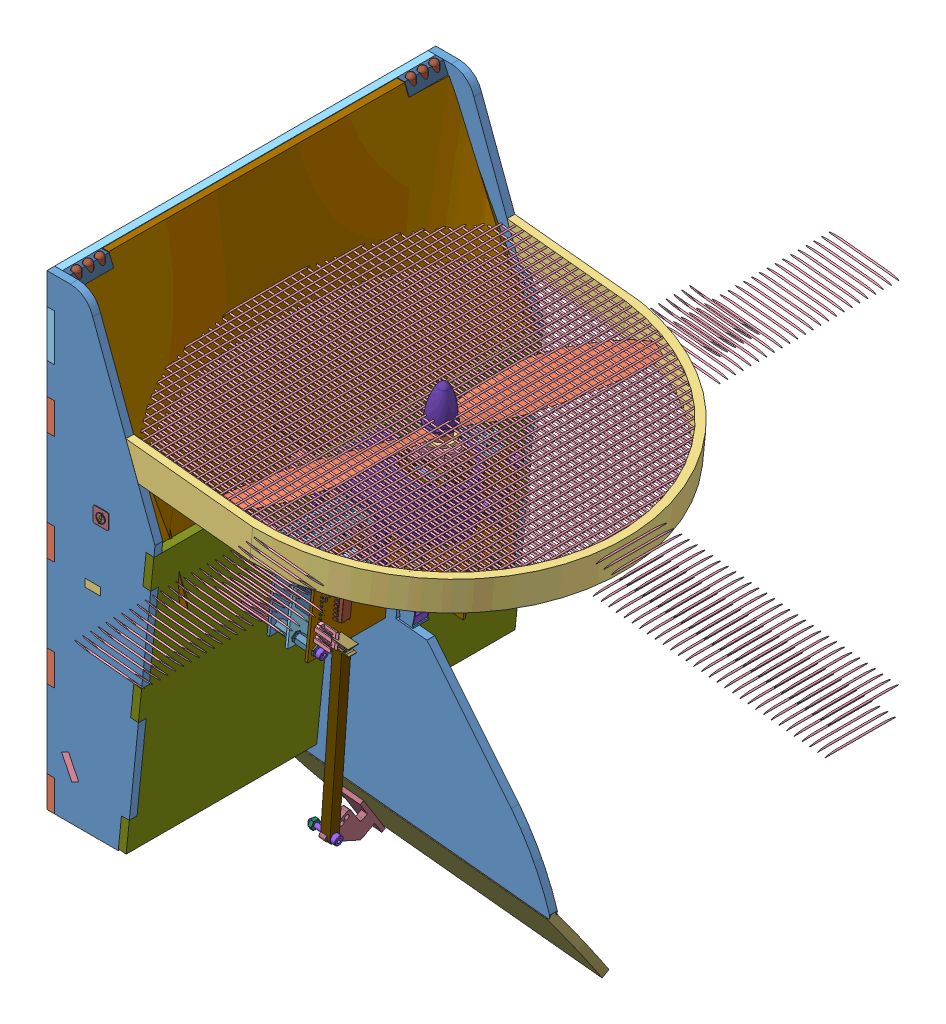
SolidWorks assembly AssTotaleSimu7, configuration Défaut. Lengths in mm. (continued)
Components (placement in the parent): (continued)
- AssStructSimu-1: AssStructSimu [Défaut] at (-125.7658 -1.8483 624.6548) x (1 0 0) z (0 0 -1) size (253.25 324.59 251.6) (continued)
  - AssCarte-1: AssCarte [Défaut] at (38.0121 147.1029 290.772) x (-0.101852 0.9948 0) z (0.9948 0.101852 0) size (66.52 130.57 98.72) (continued)
    - carte_onduleur_v3-1: carte_onduleur_v3 [Défaut] at (-131.8199 12.0892 20.7912) size (66.52 130.57 82.34) (continued)
      - RC2_2-1: RC2_2 [Défaut] at (-22 0.18 -0.803) x (-1 0 0) z (0 0 -1) size (2.34 1.04 0.5) (continued)
        - Open CASCADE STEP translator 6.8 1.12.1-1: Open CASCADE STEP translator 6.8 1.12.1 [Défaut] at origin size (2.34 1.04 0.5) (continued)
          - Pin_2_2-1: Pin_2_2 [Défaut] at origin size (0.51 1.02 0.5)
      - RC3_1-1: RC3_1 [Défaut] at (-20.9336 -14.5 -0.803) x (1 0 0) z (0 0 -1) size (2.34 1.04 0.5)
        - Open CASCADE STEP translator 6.8 1.12.1-1: Open CASCADE STEP translator 6.8 1.12.1 [Défaut] at origin size (2.34 1.04 0.5)
          - Body_1_3-1: Body_1_3 [Défaut] at origin size (2.29 1.04 0.43)
          - Pin_1_2-1: Pin_1_2 [Défaut] at (0.3048 0 0) x (-1 0 0) z (0 0 1) size (0.51 1.02 0.5)
          - Pin_2_2-1: Pin_2_2 [Défaut] at origin size (0.51 1.02 0.5)
      - RC3_2-1: RC3_2 [Défaut] at (-22.3 -14.5 -0.803) x (-1 0 0) z (0 0 -1) size (2.34 1.04 0.5)
        - Open CASCADE STEP translator 6.8 1.12.1-1: Open CASCADE STEP translator 6.8 1.12.1 [Défaut] at origin size (2.34 1.04 0.5)
          - Body_1_3-1: Body_1_3 [Défaut] at origin size (2.29 1.04 0.43)
          - Pin_1_2-1: Pin_1_2 [Défaut] at (0.3048 0 0) x (-1 0 0) z (0 0 1) size (0.51 1.02 0.5)
          - Pin_2_2-1: Pin_2_2 [Défaut] at origin size (0.51 1.02 0.5)
      - U_MES_CUR-1: U_MES_CUR [Défaut] at (-11.5 6.7816 0.803) size (2.54 2.41 0.76)
        - Open CASCADE STEP translator 6.8 1.32.1-1: Open CASCADE STEP translator 6.8 1.32.1 [Défaut] at origin size (2.54 2.41 0.76)
          - Body_1_5-1: Body_1_5 [Défaut] at origin size (2.54 1.27 0.71)
          - Pin_1_3-1: Pin_1_3 [Défaut] at (-2.1082 0.2286 0) x (0 -1 0) z (0 0 1) size (1.14 0.25 0.47)
          - Pin_2_3-1: Pin_2_3 [Défaut] at (-0.2032 2.1336 0) x (0 -1 0) z (0 0 1) size (1.14 0.25 0.47)
      - CARTE_ALIM-1: CARTE_ALIM [Défaut] at (-6.4 -57.2 0.803) size (60 130 18.35)
        - Open CASCADE STEP translator 6.8 1.33.1-1: Open CASCADE STEP translator 6.8 1.33.1 [Défaut] at origin size (60 130 18.35)
          - Body_1_6-1: Body_1_6 [Défaut] at (7 56 -12) size (60 130 18.35)
            - 1_3-1: 1_3 [Défaut] at origin size (60 130 1.61)
            - 13_3-1: 13_3 [Défaut] at (0.4717 -40.93 0.803) x (0 1 0) z (0 0 1) size (5.65 4.9 1.7)
              - =_[0_1_1_4]_3-1: =_[0_1_1_4]_3 [Défaut] at origin size (5.65 4.9 1.7)
                - 2-1: 2 [Défaut] at origin size (3.75 4.9 1.53)
                - 3-1: 3 [Défaut] at origin size (0.95 0.51 1.06)
                - 4-1: 4 [Défaut] at origin size (0.95 0.51 1.06)
                - 5_2-1: 5_2 [Défaut] at origin size (0.95 0.51 1.06)
                - 6-1: 6 [Défaut] at origin size (0.95 0.51 1.06)
                - 7-1: 7 [Défaut] at (10.8 -5.08 0) x (-1 0 0) z (0 0 1) size (0.95 0.51 1.06)
                - 8_2-1: 8_2 [Défaut] at (10.8 -2.54 0) x (-1 0 0) z (0 0 1) size (0.95 0.51 1.06)
                - 9-1: 9 [Défaut] at (10.8 0 0) x (-1 0 0) z (0 0 1) size (0.95 0.51 1.06)
                - 10-1: 10 [Défaut] at (10.8 2.54 0) x (-1 0 0) z (0 0 1) size (0.95 0.51 1.06)
                - 11_2-1: 11_2 [Défaut] at (5.4 -1.27 0) x (-1 0 0) z (0 0 1) size (4.25 2.34 1.06)
            - 18-1: 18 [Défaut] at (-2.5283 -37.23 0.803) x (0 -1 0) z (0 0 1) size (2.34 1.04 0.5)
              - =_[0_1_1_16]-1: =_[0_1_1_16] [Défaut] at origin size (2.34 1.04 0.5)
                - 14_2-1: 14_2 [Défaut] at origin size (2.29 1.04 0.43)
                - 15_2-1: 15_2 [Défaut] at (0.3048 0 0) x (-1 0 0) z (0 0 1) size (0.51 1.02 0.5)
                - 16_2-1: 16_2 [Défaut] at origin size (0.51 1.02 0.5)
            - 21_2-1: 21_2 [Défaut] at (-2.2263 -24.628 -0.803) x (1 0 0) z (0 0 -1) size (8.01 8 14.24)
              - =_[0_1_1_21]-1: =_[0_1_1_21] [Défaut] at origin size (8.01 8 14.24)
                - 19-1: 19 [Défaut] at (1.8 0 0) x (1 0 0) z (0 -1 0) size (8.01 14.24 8)
            - 23_2-1: 23_2 [Défaut] at (1.2381 -31.53 0.803) size (2.34 1.04 0.5)
              - =_[0_1_1_16]-1: =_[0_1_1_16] [Défaut] at origin size (2.34 1.04 0.5)
                - 14_2-1: 14_2 [Défaut] at origin size (2.29 1.04 0.43)
                - 15_2-1: 15_2 [Défaut] at (0.3048 0 0) x (-1 0 0) z (0 0 1) size (0.51 1.02 0.5)
                - 16_2-1: 16_2 [Défaut] at origin size (0.51 1.02 0.5)
            - 28-1: 28 [Défaut] at (5 29.8636 0.803) x (0 -1 0) z (0 0 1) size (3.35 1.3 0.55)
              - =_[0_1_1_25]_2-1: =_[0_1_1_25]_2 [Défaut] at origin size (3.35 1.3 0.55)
                - 24-1: 24 [Défaut] at origin size (3.3 1.3 0.48)
                - 25_2-1: 25_2 [Défaut] at (0.5588 0 0) x (-1 0 0) z (0 0 1) size (0.76 1.27 0.55)
                - 26_2-1: 26_2 [Défaut] at origin size (0.76 1.27 0.55)
            - 30-1: 30 [Défaut] at (6.7 29.8636 0.803) x (0 -1 0) z (0 0 1) size (2.34 1.04 0.5)
              - =_[0_1_1_16]-1: =_[0_1_1_16] [Défaut] at origin size (2.34 1.04 0.5)
                - 14_2-1: 14_2 [Défaut] at origin size (2.29 1.04 0.43)
                - 15_2-1: 15_2 [Défaut] at (0.3048 0 0) x (-1 0 0) z (0 0 1) size (0.51 1.02 0.5)
                - 16_2-1: 16_2 [Défaut] at origin size (0.51 1.02 0.5)
            - 35_2-1: 35_2 [Défaut] at (-2.5 -46.37 0.803) x (0 1 0) z (0 0 1) size (3.4 2.06 0.79)
              - =_[0_1_1_31]-1: =_[0_1_1_31] [Défaut] at origin size (3.4 2.06 0.79)
                - 31_2-1: 31_2 [Défaut] at origin size (3.3 2.06 0.69)
                - 32_3-1: 32_3 [Défaut] at (0.5588 0 0) x (-1 0 0) z (0 0 1) size (0.81 2.03 0.79)
                - 33_3-1: 33_3 [Défaut] at origin size (0.81 2.03 0.79)
            - 37-1: 37 [Défaut] at (5 31.43 0.803) x (0 1 0) z (0 0 1) size (2.34 1.04 0.5)
              - =_[0_1_1_16]-1: =_[0_1_1_16] [Défaut] at origin size (2.34 1.04 0.5)
                - 14_2-1: 14_2 [Défaut] at origin size (2.29 1.04 0.43)
                - 15_2-1: 15_2 [Défaut] at (0.3048 0 0) x (-1 0 0) z (0 0 1) size (0.51 1.02 0.5)
                - 16_2-1: 16_2 [Défaut] at origin size (0.51 1.02 0.5)
            - 39-1: 39 [Défaut] at (-0.2 35.63 0.803) x (-1 0 0) z (0 0 1) size (2.34 1.04 0.5)
              - =_[0_1_1_16]-1: =_[0_1_1_16] [Défaut] at origin size (2.34 1.04 0.5)
                - 14_2-1: 14_2 [Défaut] at origin size (2.29 1.04 0.43)
                - 15_2-1: 15_2 [Défaut] at (0.3048 0 0) x (-1 0 0) z (0 0 1) size (0.51 1.02 0.5)
                - 16_2-1: 16_2 [Défaut] at origin size (0.51 1.02 0.5)
            - 41-1: 41 [Défaut] at (2.9 -45.5036 0.803) x (0 1 0) z (0 0 1) size (2.34 1.04 0.5)
              - =_[0_1_1_16]-1: =_[0_1_1_16] [Défaut] at origin size (2.34 1.04 0.5)
                - 14_2-1: 14_2 [Défaut] at origin size (2.29 1.04 0.43)
                - 15_2-1: 15_2 [Défaut] at (0.3048 0 0) x (-1 0 0) z (0 0 1) size (0.51 1.02 0.5)
                - 16_2-1: 16_2 [Défaut] at origin size (0.51 1.02 0.5)
            - 43-1: 43 [Défaut] at (17.1348 -42.6272 0.803) x (0 1 0) z (0 0 1) size (2.34 1.04 0.5)
              - =_[0_1_1_16]-1: =_[0_1_1_16] [Défaut] at origin size (2.34 1.04 0.5)
                - 14_2-1: 14_2 [Défaut] at origin size (2.29 1.04 0.43)
                - 15_2-1: 15_2 [Défaut] at (0.3048 0 0) x (-1 0 0) z (0 0 1) size (0.51 1.02 0.5)
                - 16_2-1: 16_2 [Défaut] at origin size (0.51 1.02 0.5)
            - 48_2-1: 48_2 [Défaut] at (-5.4717 -39.01 0.803) x (-1 0 0) z (0 0 1) size (4.19 3.4 1.75)
              - =_[0_1_1_40]-1: =_[0_1_1_40] [Défaut] at origin size (4.19 3.4 1.75)
                - 44_2-1: 44_2 [Défaut] at origin size (3.75 3.38 1.73)
                - 45_2-1: 45_2 [Défaut] at (0.438 0 0) x (-1 0 0) z (0 0 1) size (0.53 3.4 1.75)
                - 46_2-1: 46_2 [Défaut] at origin size (0.52 3.4 1.75)
            - 53-1: 53 [Défaut] at (0.9 35.63 0.803) size (2.34 1.04 0.5)
              - =_[0_1_1_45]-1: =_[0_1_1_45] [Défaut] at origin size (2.34 1.04 0.5)
                - 49_3-1: 49_3 [Défaut] at origin size (2.29 1.04 0.43)
                - 50-1: 50 [Défaut] at (0.3048 0 0) x (-1 0 0) z (0 0 1) size (0.51 1.02 0.5)
                - 51-1: 51 [Défaut] at origin size (0.51 1.02 0.5)
            - 55_2-1: 55_2 [Défaut] at (1.3 -45.5036 0.803) x (0 1 0) z (0 0 1) size (2.34 1.04 0.5)
              - =_[0_1_1_45]-1: =_[0_1_1_45] [Défaut] at origin size (2.34 1.04 0.5)
                - 49_3-1: 49_3 [Défaut] at origin size (2.29 1.04 0.43)
                - 50-1: 50 [Défaut] at (0.3048 0 0) x (-1 0 0) z (0 0 1) size (0.51 1.02 0.5)
                - 51-1: 51 [Défaut] at origin size (0.51 1.02 0.5)
            - 57_3-1: 57_3 [Défaut] at (17.2348 -43.9936 0.803) x (0 -1 0) z (0 0 1) size (2.34 1.04 0.5)
              - =_[0_1_1_45]-1: =_[0_1_1_45] [Défaut] at origin size (2.34 1.04 0.5)
                - 49_3-1: 49_3 [Défaut] at origin size (2.29 1.04 0.43)
                - 50-1: 50 [Défaut] at (0.3048 0 0) x (-1 0 0) z (0 0 1) size (0.51 1.02 0.5)
                - 51-1: 51 [Défaut] at origin size (0.51 1.02 0.5)
            - 65-1: 65 [Défaut] at (-4.8 30.93 0.803) x (-1 0 0) z (0 0 1) size (14.64 9.83 4.25)
              - =_[0_1_1_52]-1: =_[0_1_1_52] [Défaut] at origin size (14.64 9.83 4.25)
                - 63_2-1: 63_2 [Défaut] at (3 0 0) x (0 -1 0) z (0 0 1) size (9.83 14.64 4.25)
                  - =_[0_1_1_3]_5-1: =_[0_1_1_3]_5 [Défaut] at origin size (9.83 9.05 4.21)
                  - =_[0_1_1_4]_5-1: =_[0_1_1_4]_5 [Défaut] at origin size (9.48 7.76 1.21)
                  - =_[0_1_1_5]_5-1: =_[0_1_1_5]_5 [Défaut] at origin size (1.36 6.01 3.08)
                  - =_[0_1_1_6]_3-1: =_[0_1_1_6]_3 [Défaut] at origin size (1.36 6.01 3.08)
                  - =_[0_1_1_7]_3-1: =_[0_1_1_7]_3 [Défaut] at origin size (1.06 6.01 3.08)
            - 67-1: 67 [Défaut] at (13.5933 -37.5272 0.803) x (-1 0 0) z (0 0 1) size (2.34 1.04 0.5)
              - =_[0_1_1_16]-1: =_[0_1_1_16] [Défaut] at origin size (2.34 1.04 0.5)
                - 14_2-1: 14_2 [Défaut] at origin size (2.29 1.04 0.43)
                - 15_2-1: 15_2 [Défaut] at (0.3048 0 0) x (-1 0 0) z (0 0 1) size (0.51 1.02 0.5)
                - 16_2-1: 16_2 [Défaut] at origin size (0.51 1.02 0.5)
            - 70_2-1: 70_2 [Défaut] at (18.2733 -29.7272 0.803) x (0 1 0) z (0 0 1) size (6.06 4.95 1.88)
              - =_[0_1_1_61]-1: =_[0_1_1_61] [Défaut] at origin size (6.06 4.95 1.88)
                - 68-1: 68 [Défaut] x (1 0 0) z (0 -1 0) size (6.06 1.88 4.95)
            - 83-1: 83 [Défaut] at (-21.2 -38.07 0.803) x (-1 0 0) z (0 0 1) size (2.7 5.2 1.11)
              - =_[0_1_1_64]-1: =_[0_1_1_64] [Défaut] at origin size (2.7 5.2 1.11)
                - 84_2-1: 84_2 [Défaut] at (1.2 -4 0) x (0 1 0) z (0 0 1) size (5.2 2.7 1.11)
                  - =_[0_1_1_3]_6-1: =_[0_1_1_3]_6 [Défaut] at origin size (0.39 0.64 0.01)
                  - =_[0_1_1_4]_6-1: =_[0_1_1_4]_6 [Défaut] at origin size (0.6 1.9 0.2)
                  - =_[0_1_1_5]_6-1: =_[0_1_1_5]_6 [Défaut] at origin size (0.21 0.08 0.01)
                  - =_[0_1_1_6]_4-1: =_[0_1_1_6]_4 [Défaut] at origin size (0.6 1.9 0.2)
                  - =_[0_1_1_7]_4-1: =_[0_1_1_7]_4 [Défaut] at origin size (0.46 0.68 0.01)
                  - =_[0_1_1_8]_3-1: =_[0_1_1_8]_3 [Défaut] at origin size (0.38 0.66 0.01)
                  - =_[0_1_1_9]_2-1: =_[0_1_1_9]_2 [Défaut] at origin size (0.2 0.62 0.01)
                  - =_[0_1_1_10]_2-1: =_[0_1_1_10]_2 [Défaut] at origin size (4 2.7 1.1)
                  - =_[0_1_1_11]_2-1: =_[0_1_1_11]_2 [Défaut] at origin size (0.46 0.63 0.01)
                  - =_[0_1_1_12]_2-1: =_[0_1_1_12]_2 [Défaut] at origin size (0.56 0.68 0.01)
            - 86_2-1: 86_2 [Défaut] at (12.8933 -35.4272 0.803) x (0 1 0) z (0 0 1) size (2.7 5.2 1.11)
              - =_[0_1_1_77]-1: =_[0_1_1_77] [Défaut] at origin size (2.7 5.2 1.11)
                - 84_2-1: 84_2 [Défaut] at (1.2 -4 0) x (0 1 0) z (0 0 1) size (5.2 2.7 1.11)
                  - =_[0_1_1_3]_6-1: =_[0_1_1_3]_6 [Défaut] at origin size (0.39 0.64 0.01)
                  - =_[0_1_1_4]_6-1: =_[0_1_1_4]_6 [Défaut] at origin size (0.6 1.9 0.2)
                  - =_[0_1_1_5]_6-1: =_[0_1_1_5]_6 [Défaut] at origin size (0.21 0.08 0.01)
                  - =_[0_1_1_6]_4-1: =_[0_1_1_6]_4 [Défaut] at origin size (0.6 1.9 0.2)
                  - =_[0_1_1_7]_4-1: =_[0_1_1_7]_4 [Défaut] at origin size (0.46 0.68 0.01)
                  - =_[0_1_1_8]_3-1: =_[0_1_1_8]_3 [Défaut] at origin size (0.38 0.66 0.01)
                  - =_[0_1_1_9]_2-1: =_[0_1_1_9]_2 [Défaut] at origin size (0.2 0.62 0.01)
                  - =_[0_1_1_10]_2-1: =_[0_1_1_10]_2 [Défaut] at origin size (4 2.7 1.1)
                  - =_[0_1_1_11]_2-1: =_[0_1_1_11]_2 [Défaut] at origin size (0.46 0.63 0.01)
                  - =_[0_1_1_12]_2-1: =_[0_1_1_12]_2 [Défaut] at origin size (0.56 0.68 0.01)
            - 92_2-1: 92_2 [Défaut] at (20.9933 -39.3272 0.803) x (0 -1 0) z (0 0 1) size (2.79 1.98 0.64)
              - =_[0_1_1_79]-1: =_[0_1_1_79] [Défaut] at origin size (2.79 1.98 0.64)
                - 87-1: 87 [Défaut] at origin size (2.79 1.02 0.58)
                - 88-1: 88 [Défaut] x (0 -1 0) z (0 0 1) size (0.42 0.38 0.38)
                - 89-1: 89 [Défaut] at (-2.8448 -0.9652 0) x (0 1 0) z (0 0 1) size (0.55 0.38 0.38)
                - 90-1: 90 [Défaut] at (-0.9652 -2.8448 0) x (0 1 0) z (0 0 1) size (0.55 0.38 0.38)
            - 98-1: 98 [Défaut] at (-17.7 -48.47 0.803) x (0 -1 0) z (0 0 1) size (2.54 1.98 0.64)
              - =_[0_1_1_85]-1: =_[0_1_1_85] [Défaut] at origin size (2.54 1.98 0.64)
                - 93-1: 93 [Défaut] at origin size (2.54 1.14 0.58)
                - 94-1: 94 [Défaut] x (0 -1 0) z (0 0 1) size (0.43 0.51 0.38)
                - 95-1: 95 [Défaut] at (1.8796 1.8796 0) x (0 -1 0) z (0 0 1) size (0.43 0.51 0.38)
                - 96-1: 96 [Défaut] at (-0.9652 -2.8448 0) x (0 1 0) z (0 0 1) size (0.41 0.51 0.38)
            - 100-1: 100 [Défaut] at (24.3933 -43.2272 0.803) size (2.79 1.98 0.64)
              - =_[0_1_1_79]-1: =_[0_1_1_79] [Défaut] at origin size (2.79 1.98 0.64)
                - 87-1: 87 [Défaut] at origin size (2.79 1.02 0.58)
                - 88-1: 88 [Défaut] x (0 -1 0) z (0 0 1) size (0.42 0.38 0.38)
                - 89-1: 89 [Défaut] at (-2.8448 -0.9652 0) x (0 1 0) z (0 0 1) size (0.55 0.38 0.38)
                - 90-1: 90 [Défaut] at (-0.9652 -2.8448 0) x (0 1 0) z (0 0 1) size (0.55 0.38 0.38)
            - 102-1: 102 [Défaut] at (21.4933 -44.4272 0.803) x (0 -1 0) z (0 0 1) size (2.79 1.98 0.64)
              - =_[0_1_1_79]-1: =_[0_1_1_79] [Défaut] at origin size (2.79 1.98 0.64)
                - 87-1: 87 [Défaut] at origin size (2.79 1.02 0.58)
                - 88-1: 88 [Défaut] x (0 -1 0) z (0 0 1) size (0.42 0.38 0.38)
                - 89-1: 89 [Défaut] at (-2.8448 -0.9652 0) x (0 1 0) z (0 0 1) size (0.55 0.38 0.38)
                - 90-1: 90 [Défaut] at (-0.9652 -2.8448 0) x (0 1 0) z (0 0 1) size (0.55 0.38 0.38)
            - 107-1: 107 [Défaut] at (23.1933 -29.1272 -0.803) x (0 1 0) z (0 0 -1) size (9.6 14.35 5)
              - =_[0_1_1_93]-1: =_[0_1_1_93] [Défaut] at origin size (9.6 14.35 5)
                - 105-1: 105 [Défaut] at (0.5 -1 2) x (-1 0 0) z (0 0 1) size (9.6 14.35 5)
                  - =_[0_1_1_3]_7-1: =_[0_1_1_3]_7 [Défaut] at origin size (9.6 12.75 5)
                  - =_[0_1_1_4]_7-1: =_[0_1_1_4]_7 [Défaut] at origin size (2.2 1.6 2.2)
            - 109-1: 109 [Défaut] at (25.4933 -41.1272 0.803) x (-1 0 0) z (0 0 1) size (2.34 1.04 0.5)
              - =_[0_1_1_45]-1: =_[0_1_1_45] [Défaut] at origin size (2.34 1.04 0.5)
                - 49_3-1: 49_3 [Défaut] at origin size (2.29 1.04 0.43)
                - 50-1: 50 [Défaut] at (0.3048 0 0) x (-1 0 0) z (0 0 1) size (0.51 1.02 0.5)
                - 51-1: 51 [Défaut] at origin size (0.51 1.02 0.5)
            - 111-1: 111 [Défaut] at (22.0269 -41.8272 0.803) x (-1 0 0) z (0 0 1) size (2.34 1.04 0.5)
              - =_[0_1_1_45]-1: =_[0_1_1_45] [Défaut] at origin size (2.34 1.04 0.5)
                - 49_3-1: 49_3 [Défaut] at origin size (2.29 1.04 0.43)
                - 50-1: 50 [Défaut] at (0.3048 0 0) x (-1 0 0) z (0 0 1) size (0.51 1.02 0.5)
                - 51-1: 51 [Défaut] at origin size (0.51 1.02 0.5)
            - 113-1: 113 [Défaut] at (-24.8 -36.7036 0.803) x (0 1 0) z (0 0 1) size (2.34 1.04 0.5)
              - =_[0_1_1_45]-1: =_[0_1_1_45] [Défaut] at origin size (2.34 1.04 0.5)
                - 49_3-1: 49_3 [Défaut] at origin size (2.29 1.04 0.43)
                - 50-1: 50 [Défaut] at (0.3048 0 0) x (-1 0 0) z (0 0 1) size (0.51 1.02 0.5)
                - 51-1: 51 [Défaut] at origin size (0.51 1.02 0.5)
            - 115-1: 115 [Défaut] at (-24.8 -40.3036 0.803) x (0 1 0) z (0 0 1) size (2.34 1.04 0.5)
              - =_[0_1_1_45]-1: =_[0_1_1_45] [Défaut] at origin size (2.34 1.04 0.5)
                - 49_3-1: 49_3 [Défaut] at origin size (2.29 1.04 0.43)
                - 50-1: 50 [Défaut] at (0.3048 0 0) x (-1 0 0) z (0 0 1) size (0.51 1.02 0.5)
                - 51-1: 51 [Défaut] at origin size (0.51 1.02 0.5)
            - 117-1: 117 [Défaut] at (-16 -48.27 0.803) x (0 -1 0) z (0 0 1) size (2.34 1.04 0.5)
              - =_[0_1_1_45]-1: =_[0_1_1_45] [Défaut] at origin size (2.34 1.04 0.5)
                - 49_3-1: 49_3 [Défaut] at origin size (2.29 1.04 0.43)
                - 50-1: 50 [Défaut] at (0.3048 0 0) x (-1 0 0) z (0 0 1) size (0.51 1.02 0.5)
                - 51-1: 51 [Défaut] at origin size (0.51 1.02 0.5)
            - 119-1: 119 [Défaut] at (-22.5189 -47.87 0.803) x (-1 0 0) z (0 0 1) size (2.34 1.04 0.5)
              - =_[0_1_1_45]-1: =_[0_1_1_45] [Défaut] at origin size (2.34 1.04 0.5)
                - 49_3-1: 49_3 [Défaut] at origin size (2.29 1.04 0.43)
                - 50-1: 50 [Défaut] at (0.3048 0 0) x (-1 0 0) z (0 0 1) size (0.51 1.02 0.5)
                - 51-1: 51 [Défaut] at origin size (0.51 1.02 0.5)
            - 121-1: 121 [Défaut] at (22.3933 -38.9272 0.803) size (2.34 1.04 0.5)
              - =_[0_1_1_45]-1: =_[0_1_1_45] [Défaut] at origin size (2.34 1.04 0.5)
                - 49_3-1: 49_3 [Défaut] at origin size (2.29 1.04 0.43)
                - 50-1: 50 [Défaut] at (0.3048 0 0) x (-1 0 0) z (0 0 1) size (0.51 1.02 0.5)
                - 51-1: 51 [Défaut] at origin size (0.51 1.02 0.5)
            - 123-1: 123 [Défaut] at (22.0933 -36.4272 0.803) x (-1 0 0) z (0 0 1) size (2.34 1.04 0.5)
              - =_[0_1_1_45]-1: =_[0_1_1_45] [Défaut] at origin size (2.34 1.04 0.5)
                - 49_3-1: 49_3 [Défaut] at origin size (2.29 1.04 0.43)
                - 50-1: 50 [Défaut] at (0.3048 0 0) x (-1 0 0) z (0 0 1) size (0.51 1.02 0.5)
                - 51-1: 51 [Défaut] at origin size (0.51 1.02 0.5)
            - 125-1: 125 [Défaut] at (22.3933 -32.0272 0.803) x (0 -1 0) z (0 0 1) size (2.34 1.04 0.5)
              - =_[0_1_1_45]-1: =_[0_1_1_45] [Défaut] at origin size (2.34 1.04 0.5)
                - 49_3-1: 49_3 [Défaut] at origin size (2.29 1.04 0.43)
                - 50-1: 50 [Défaut] at (0.3048 0 0) x (-1 0 0) z (0 0 1) size (0.51 1.02 0.5)
                - 51-1: 51 [Défaut] at origin size (0.51 1.02 0.5)
            - 127-1: 127 [Défaut] at (17.9597 -23.1272 0.803) size (2.34 1.04 0.5)
              - =_[0_1_1_16]-1: =_[0_1_1_16] [Défaut] at origin size (2.34 1.04 0.5)
                - 14_2-1: 14_2 [Défaut] at origin size (2.29 1.04 0.43)
                - 15_2-1: 15_2 [Défaut] at (0.3048 0 0) x (-1 0 0) z (0 0 1) size (0.51 1.02 0.5)
                - 16_2-1: 16_2 [Défaut] at origin size (0.51 1.02 0.5)
            - 129-1: 129 [Défaut] at (20.0269 -24.9272 0.803) x (-1 0 0) z (0 0 1) size (2.34 1.04 0.5)
              - =_[0_1_1_16]-1: =_[0_1_1_16] [Défaut] at origin size (2.34 1.04 0.5)
                - 14_2-1: 14_2 [Défaut] at origin size (2.29 1.04 0.43)
                - 15_2-1: 15_2 [Défaut] at (0.3048 0 0) x (-1 0 0) z (0 0 1) size (0.51 1.02 0.5)
                - 16_2-1: 16_2 [Défaut] at origin size (0.51 1.02 0.5)
            - 131-1: 131 [Défaut] at (16.9933 -37.5272 0.803) x (-1 0 0) z (0 0 1) size (2.34 1.04 0.5)
              - =_[0_1_1_45]-1: =_[0_1_1_45] [Défaut] at origin size (2.34 1.04 0.5)
                - 49_3-1: 49_3 [Défaut] at origin size (2.29 1.04 0.43)
                - 50-1: 50 [Défaut] at (0.3048 0 0) x (-1 0 0) z (0 0 1) size (0.51 1.02 0.5)
                - 51-1: 51 [Défaut] at origin size (0.51 1.02 0.5)
            - 136-1: 136 [Défaut] at (3.2957 -29.23 0.803) x (-1 0 0) z (0 0 1) size (4.78 2.79 2.03)
              - =_[0_1_1_110]_2-1: =_[0_1_1_110]_2 [Défaut] at origin size (4.78 2.79 2.03)
                - 132-1: 132 [Défaut] at origin size (4.32 2.79 1.78)
                - 133-1: 133 [Défaut] at (0.4572 0 0) x (-1 0 0) z (0 0 1) size (1.02 1.27 1.32)
                - 134-1: 134 [Défaut] at origin size (1.02 1.27 1.32)
            - 141-1: 141 [Défaut] at (0.2436 -33.3673 0.803) size (3.35 1.3 0.55)
              - =_[0_1_1_115]_2-1: =_[0_1_1_115]_2 [Défaut] at origin size (3.35 1.3 0.55)
                - 137-1: 137 [Défaut] at origin size (3.3 1.3 0.48)
                - 138-1: 138 [Défaut] at (0.5588 0 0) x (-1 0 0) z (0 0 1) size (0.76 1.27 0.55)
                - 139-1: 139 [Défaut] at origin size (0.76 1.27 0.55)
            - 143_2-1: 143_2 [Défaut] at (-0.3 -45.47 0.803) x (0 1 0) z (0 0 1) size (2.34 1.04 0.5)
              - =_[0_1_1_16]-1: =_[0_1_1_16] [Défaut] at origin size (2.34 1.04 0.5)
                - 14_2-1: 14_2 [Défaut] at origin size (2.29 1.04 0.43)
                - 15_2-1: 15_2 [Défaut] at (0.3048 0 0) x (-1 0 0) z (0 0 1) size (0.51 1.02 0.5)
                - 16_2-1: 16_2 [Défaut] at origin size (0.51 1.02 0.5)
            - 145-1: 145 [Défaut] at (6.6 31.13 0.803) x (0 1 0) z (0 0 1) size (3.35 1.3 0.55)
              - =_[0_1_1_25]_2-1: =_[0_1_1_25]_2 [Défaut] at origin size (3.35 1.3 0.55)
                - 24-1: 24 [Défaut] at origin size (3.3 1.3 0.48)
                - 25_2-1: 25_2 [Défaut] at (0.5588 0 0) x (-1 0 0) z (0 0 1) size (0.76 1.27 0.55)
                - 26_2-1: 26_2 [Défaut] at origin size (0.76 1.27 0.55)
            - 148-1: 148 [Défaut] at (-7.5 -56.57 0.803) size (15.24 2.54 7.37)
              - =_[0_1_1_122]_2-1: =_[0_1_1_122]_2 [Défaut] at origin size (15.24 2.54 7.37)
                - 146-1: 146 [Défaut] at (6.3 0 1) x (1 0 0) z (0 -1 0) size (15.24 7.37 2.54)
      - COMP1-1: COMP1 [Défaut] at (-16.3 -36.2 0.803) x (-1 0 0) z (0 0 1) size (2.03 1.88 0.51)
        - Open CASCADE STEP translator 6.8 1.34.1-1: Open CASCADE STEP translator 6.8 1.34.1 [Défaut] at origin size (2.03 1.88 0.51)
          - Body_1_6-1: Body_1_6 [Défaut] at origin size (2.03 1.02 0.46)
          - Pin_1_4-1: Pin_1_4 [Défaut] x (0 1 0) z (0 0 1) size (0.45 0.25 0.32)
          - Pin_2_4-1: Pin_2_4 [Défaut] at (0.65 -0.65 0) x (0 1 0) z (0 0 1) size (0.45 0.25 0.32)
          - Pin_3-1: Pin_3 [Défaut] at (1.3 -1.3 0) x (0 1 0) z (0 0 1) size (0.45 0.25 0.32)
          - Pin_4-1: Pin_4 [Défaut] at (-0.5 3.1 0) x (0 -1 0) z (0 0 1) size (0.41 0.25 0.32)
          - Pin_5-1: Pin_5 [Défaut] at (-1.8 1.8 0) x (0 -1 0) z (0 0 1) size (0.41 0.25 0.32)
      - COMP2-1: COMP2 [Défaut] at (-14.3 -9.6 0.803) x (-1 0 0) z (0 0 1) size (2.03 1.88 0.51)
        - Open CASCADE STEP translator 6.8 1.34.1-1: Open CASCADE STEP translator 6.8 1.34.1 [Défaut] at origin size (2.03 1.88 0.51)
          - Body_1_6-1: Body_1_6 [Défaut] at origin size (2.03 1.02 0.46)
          - Pin_1_4-1: Pin_1_4 [Défaut] x (0 1 0) z (0 0 1) size (0.45 0.25 0.32)
          - Pin_2_4-1: Pin_2_4 [Défaut] at (0.65 -0.65 0) x (0 1 0) z (0 0 1) size (0.45 0.25 0.32)
          - Pin_3-1: Pin_3 [Défaut] at (1.3 -1.3 0) x (0 1 0) z (0 0 1) size (0.45 0.25 0.32)
          - Pin_4-1: Pin_4 [Défaut] at (-0.5 3.1 0) x (0 -1 0) z (0 0 1) size (0.41 0.25 0.32)
          - Pin_5-1: Pin_5 [Défaut] at (-1.8 1.8 0) x (0 -1 0) z (0 0 1) size (0.41 0.25 0.32)
      - COMP3-1: COMP3 [Défaut] at (-15.9 -23.2 0.803) x (-1 0 0) z (0 0 1) size (2.03 1.88 0.51)
        - Open CASCADE STEP translator 6.8 1.34.1-1: Open CASCADE STEP translator 6.8 1.34.1 [Défaut] at origin size (2.03 1.88 0.51)
          - Body_1_6-1: Body_1_6 [Défaut] at origin size (2.03 1.02 0.46)
          - Pin_1_4-1: Pin_1_4 [Défaut] x (0 1 0) z (0 0 1) size (0.45 0.25 0.32)
          - Pin_2_4-1: Pin_2_4 [Défaut] at (0.65 -0.65 0) x (0 1 0) z (0 0 1) size (0.45 0.25 0.32)
          - Pin_3-1: Pin_3 [Défaut] at (1.3 -1.3 0) x (0 1 0) z (0 0 1) size (0.45 0.25 0.32)
          - Pin_4-1: Pin_4 [Défaut] at (-0.5 3.1 0) x (0 -1 0) z (0 0 1) size (0.41 0.25 0.32)
          - Pin_5-1: Pin_5 [Défaut] at (-1.8 1.8 0) x (0 -1 0) z (0 0 1) size (0.41 0.25 0.32)
      - CP1-1: CP1 [Défaut] at (-18.9 -38.2 0.803) x (0 1 0) z (0 0 1) size (2.34 1.04 0.5)
        - Open CASCADE STEP translator 6.8 1.6.1-1: Open CASCADE STEP translator 6.8 1.6.1 [Défaut] at origin size (2.34 1.04 0.5)
          - Body_1-1: Body_1 [Défaut] at origin size (2.29 1.04 0.43)
          - Pin_1-1: Pin_1 [Défaut] at (0.3048 0 0) x (-1 0 0) z (0 0 1) size (0.51 1.02 0.5)
          - Pin_2-1: Pin_2 [Défaut] at origin size (0.51 1.02 0.5)
      - CP2-1: CP2 [Défaut] at (-16.9 -11.6 0.803) x (0 1 0) z (0 0 1) size (2.34 1.04 0.5)
        - Open CASCADE STEP translator 6.8 1.6.1-1: Open CASCADE STEP translator 6.8 1.6.1 [Défaut] at origin size (2.34 1.04 0.5)
          - Body_1-1: Body_1 [Défaut] at origin size (2.29 1.04 0.43)
          - Pin_1-1: Pin_1 [Défaut] at (0.3048 0 0) x (-1 0 0) z (0 0 1) size (0.51 1.02 0.5)
          - Pin_2-1: Pin_2 [Défaut] at origin size (0.51 1.02 0.5)
      - CP3-1: CP3 [Défaut] at (-18.5 -25.2 0.803) x (0 1 0) z (0 0 1) size (2.34 1.04 0.5)
        - Open CASCADE STEP translator 6.8 1.6.1-1: Open CASCADE STEP translator 6.8 1.6.1 [Défaut] at origin size (2.34 1.04 0.5)
          - Body_1-1: Body_1 [Défaut] at origin size (2.29 1.04 0.43)
          - Pin_1-1: Pin_1 [Défaut] at (0.3048 0 0) x (-1 0 0) z (0 0 1) size (0.51 1.02 0.5)
          - Pin_2-1: Pin_2 [Défaut] at origin size (0.51 1.02 0.5)
      - C_DEC_COM1-1: C_DEC_COM1 [Défaut] at (-15 -36 0.803) x (0 -1 0) z (0 0 1) size (2.34 1.04 0.5)
        - Open CASCADE STEP translator 6.8 1.6.1-1: Open CASCADE STEP translator 6.8 1.6.1 [Défaut] at origin size (2.34 1.04 0.5)
          - Body_1-1: Body_1 [Défaut] at origin size (2.29 1.04 0.43)
          - Pin_1-1: Pin_1 [Défaut] at (0.3048 0 0) x (-1 0 0) z (0 0 1) size (0.51 1.02 0.5)
          - Pin_2-1: Pin_2 [Défaut] at origin size (0.51 1.02 0.5)
      - C_DEC_COMP2-1: C_DEC_COMP2 [Défaut] at (-13 -9.3 0.803) x (0 -1 0) z (0 0 1) size (2.34 1.04 0.5)
        - Open CASCADE STEP translator 6.8 1.6.1-1: Open CASCADE STEP translator 6.8 1.6.1 [Défaut] at origin size (2.34 1.04 0.5)
          - Body_1-1: Body_1 [Défaut] at origin size (2.29 1.04 0.43)
          - Pin_1-1: Pin_1 [Défaut] at (0.3048 0 0) x (-1 0 0) z (0 0 1) size (0.51 1.02 0.5)
          - Pin_2-1: Pin_2 [Défaut] at origin size (0.51 1.02 0.5)
      - C_DEC_COMP3-1: C_DEC_COMP3 [Défaut] at (-14.6 -22.9 0.803) x (0 -1 0) z (0 0 1) size (2.34 1.04 0.5)
        - Open CASCADE STEP translator 6.8 1.6.1-1: Open CASCADE STEP translator 6.8 1.6.1 [Défaut] at origin size (2.34 1.04 0.5)
          - Body_1-1: Body_1 [Défaut] at origin size (2.29 1.04 0.43)
          - Pin_1-1: Pin_1 [Défaut] at (0.3048 0 0) x (-1 0 0) z (0 0 1) size (0.51 1.02 0.5)
          - Pin_2-1: Pin_2 [Défaut] at origin size (0.51 1.02 0.5)
      - D_VBAT-1: D_VBAT [Défaut] at (-1.2 46.4 0.803) x (0 -1 0) z (0 0 1) size (2.34 1.04 0.5)
        - Open CASCADE STEP translator 6.8 1.6.1-1: Open CASCADE STEP translator 6.8 1.6.1 [Défaut] at origin size (2.34 1.04 0.5)
          - Body_1-1: Body_1 [Défaut] at origin size (2.29 1.04 0.43)
          - Pin_1-1: Pin_1 [Défaut] at (0.3048 0 0) x (-1 0 0) z (0 0 1) size (0.51 1.02 0.5)
          - Pin_2-1: Pin_2 [Défaut] at origin size (0.51 1.02 0.5)
      - D_3V-1: D_3V [Défaut] at (1.3 46.3 0.803) x (0 -1 0) z (0 0 1) size (2.34 1.04 0.5)
        - Open CASCADE STEP translator 6.8 1.6.1-1: Open CASCADE STEP translator 6.8 1.6.1 [Défaut] at origin size (2.34 1.04 0.5)
          - Body_1-1: Body_1 [Défaut] at origin size (2.29 1.04 0.43)
          - Pin_1-1: Pin_1 [Défaut] at (0.3048 0 0) x (-1 0 0) z (0 0 1) size (0.51 1.02 0.5)
          - Pin_2-1: Pin_2 [Défaut] at origin size (0.51 1.02 0.5)
      - D_5V-1: D_5V [Défaut] at (-3.7 46.4 0.803) x (0 -1 0) z (0 0 1) size (2.34 1.04 0.5)
        - Open CASCADE STEP translator 6.8 1.6.1-1: Open CASCADE STEP translator 6.8 1.6.1 [Défaut] at origin size (2.34 1.04 0.5)
          - Body_1-1: Body_1 [Défaut] at origin size (2.29 1.04 0.43)
          - Pin_1-1: Pin_1 [Défaut] at (0.3048 0 0) x (-1 0 0) z (0 0 1) size (0.51 1.02 0.5)
          - Pin_2-1: Pin_2 [Défaut] at origin size (0.51 1.02 0.5)
      - R1_1-1: R1_1 [Défaut] at (-20.2 -36.1 0.803) x (-1 0 0) z (0 0 1) size (2.34 1.04 0.5)
        - Open CASCADE STEP translator 6.8 1.12.1-1: Open CASCADE STEP translator 6.8 1.12.1 [Défaut] at origin size (2.34 1.04 0.5)
          - Body_1_3-1: Body_1_3 [Défaut] at origin size (2.29 1.04 0.43)
          - Pin_1_2-1: Pin_1_2 [Défaut] at (0.3048 0 0) x (-1 0 0) z (0 0 1) size (0.51 1.02 0.5)
          - Pin_2_2-1: Pin_2_2 [Défaut] at origin size (0.51 1.02 0.5)
      - R1_2-1: R1_2 [Défaut] at (-15.5 -34.6 0.803) x (-1 0 0) z (0 0 1) size (2.34 1.04 0.5)
        - Open CASCADE STEP translator 6.8 1.12.1-1: Open CASCADE STEP translator 6.8 1.12.1 [Défaut] at origin size (2.34 1.04 0.5)
          - Body_1_3-1: Body_1_3 [Défaut] at origin size (2.29 1.04 0.43)
          - Pin_1_2-1: Pin_1_2 [Défaut] at (0.3048 0 0) x (-1 0 0) z (0 0 1) size (0.51 1.02 0.5)
          - Pin_2_2-1: Pin_2_2 [Défaut] at origin size (0.51 1.02 0.5)
      - R1_3-1: R1_3 [Défaut] at (-20.3 -39.9 0.803) x (-1 0 0) z (0 0 1) size (2.34 1.04 0.5)
        - Open CASCADE STEP translator 6.8 1.12.1-1: Open CASCADE STEP translator 6.8 1.12.1 [Défaut] at origin size (2.34 1.04 0.5)
          - Body_1_3-1: Body_1_3 [Défaut] at origin size (2.29 1.04 0.43)
          - Pin_1_2-1: Pin_1_2 [Défaut] at (0.3048 0 0) x (-1 0 0) z (0 0 1) size (0.51 1.02 0.5)
          - Pin_2_2-1: Pin_2_2 [Défaut] at origin size (0.51 1.02 0.5)
      - R1_4-1: R1_4 [Défaut] at (-20.3 -38.1 0.803) x (-1 0 0) z (0 0 1) size (2.34 1.04 0.5)
        - Open CASCADE STEP translator 6.8 1.12.1-1: Open CASCADE STEP translator 6.8 1.12.1 [Défaut] at origin size (2.34 1.04 0.5)
          - Body_1_3-1: Body_1_3 [Défaut] at origin size (2.29 1.04 0.43)
          - Pin_1_2-1: Pin_1_2 [Défaut] at (0.3048 0 0) x (-1 0 0) z (0 0 1) size (0.51 1.02 0.5)
          - Pin_2_2-1: Pin_2_2 [Défaut] at origin size (0.51 1.02 0.5)
      - R1_5-1: R1_5 [Défaut] at (-17.1336 -39.7 0.803) size (2.34 1.04 0.5)
        - Open CASCADE STEP translator 6.8 1.12.1-1: Open CASCADE STEP translator 6.8 1.12.1 [Défaut] at origin size (2.34 1.04 0.5)
          - Body_1_3-1: Body_1_3 [Défaut] at origin size (2.29 1.04 0.43)
          - Pin_1_2-1: Pin_1_2 [Défaut] at (0.3048 0 0) x (-1 0 0) z (0 0 1) size (0.51 1.02 0.5)
          - Pin_2_2-1: Pin_2_2 [Défaut] at origin size (0.51 1.02 0.5)
      - R2_1-1: R2_1 [Défaut] at (-18.5 -9.5 0.803) x (-1 0 0) z (0 0 1) size (2.34 1.04 0.5)
        - Open CASCADE STEP translator 6.8 1.12.1-1: Open CASCADE STEP translator 6.8 1.12.1 [Défaut] at origin size (2.34 1.04 0.5)
          - Body_1_3-1: Body_1_3 [Défaut] at origin size (2.29 1.04 0.43)
          - Pin_1_2-1: Pin_1_2 [Défaut] at (0.3048 0 0) x (-1 0 0) z (0 0 1) size (0.51 1.02 0.5)
          - Pin_2_2-1: Pin_2_2 [Défaut] at origin size (0.51 1.02 0.5)
      - R2_2-1: R2_2 [Défaut] at (-13.1 -8 0.803) x (-1 0 0) z (0 0 1) size (2.34 1.04 0.5)
        - Open CASCADE STEP translator 6.8 1.12.1-1: Open CASCADE STEP translator 6.8 1.12.1 [Défaut] at origin size (2.34 1.04 0.5)
          - Body_1_3-1: Body_1_3 [Défaut] at origin size (2.29 1.04 0.43)
          - Pin_1_2-1: Pin_1_2 [Défaut] at (0.3048 0 0) x (-1 0 0) z (0 0 1) size (0.51 1.02 0.5)
          - Pin_2_2-1: Pin_2_2 [Défaut] at origin size (0.51 1.02 0.5)
      - R2_3-1: R2_3 [Défaut] at (-18.5 -11.2 0.803) x (-1 0 0) z (0 0 1) size (2.34 1.04 0.5)
        - Open CASCADE STEP translator 6.8 1.12.1-1: Open CASCADE STEP translator 6.8 1.12.1 [Défaut] at origin size (2.34 1.04 0.5)
          - Body_1_3-1: Body_1_3 [Défaut] at origin size (2.29 1.04 0.43)
          - Pin_1_2-1: Pin_1_2 [Défaut] at (0.3048 0 0) x (-1 0 0) z (0 0 1) size (0.51 1.02 0.5)
          - Pin_2_2-1: Pin_2_2 [Défaut] at origin size (0.51 1.02 0.5)
      - R2_4-1: R2_4 [Défaut] at (-18.5 -12.8 0.803) x (-1 0 0) z (0 0 1) size (2.34 1.04 0.5)
        - Open CASCADE STEP translator 6.8 1.12.1-1: Open CASCADE STEP translator 6.8 1.12.1 [Défaut] at origin size (2.34 1.04 0.5)
          - Body_1_3-1: Body_1_3 [Défaut] at origin size (2.29 1.04 0.43)
          - Pin_1_2-1: Pin_1_2 [Défaut] at (0.3048 0 0) x (-1 0 0) z (0 0 1) size (0.51 1.02 0.5)
          - Pin_2_2-1: Pin_2_2 [Défaut] at origin size (0.51 1.02 0.5)
      - R2_5-1: R2_5 [Défaut] at (-15.1336 -13 0.803) size (2.34 1.04 0.5)
        - Open CASCADE STEP translator 6.8 1.12.1-1: Open CASCADE STEP translator 6.8 1.12.1 [Défaut] at origin size (2.34 1.04 0.5)
          - Body_1_3-1: Body_1_3 [Défaut] at origin size (2.29 1.04 0.43)
          - Pin_1_2-1: Pin_1_2 [Défaut] at (0.3048 0 0) x (-1 0 0) z (0 0 1) size (0.51 1.02 0.5)
          - Pin_2_2-1: Pin_2_2 [Défaut] at origin size (0.51 1.02 0.5)
      - R3_1-1: R3_1 [Défaut] at (-19.9 -23.1 0.803) x (-1 0 0) z (0 0 1) size (2.34 1.04 0.5)
        - Open CASCADE STEP translator 6.8 1.12.1-1: Open CASCADE STEP translator 6.8 1.12.1 [Défaut] at origin size (2.34 1.04 0.5)
          - Body_1_3-1: Body_1_3 [Défaut] at origin size (2.29 1.04 0.43)
          - Pin_1_2-1: Pin_1_2 [Défaut] at (0.3048 0 0) x (-1 0 0) z (0 0 1) size (0.51 1.02 0.5)
          - Pin_2_2-1: Pin_2_2 [Défaut] at origin size (0.51 1.02 0.5)
      - R3_2-1: R3_2 [Défaut] at (-14.7 -21.6 0.803) x (-1 0 0) z (0 0 1) size (2.34 1.04 0.5)
        - Open CASCADE STEP translator 6.8 1.12.1-1: Open CASCADE STEP translator 6.8 1.12.1 [Défaut] at origin size (2.34 1.04 0.5)
          - Body_1_3-1: Body_1_3 [Défaut] at origin size (2.29 1.04 0.43)
          - Pin_1_2-1: Pin_1_2 [Défaut] at (0.3048 0 0) x (-1 0 0) z (0 0 1) size (0.51 1.02 0.5)
          - Pin_2_2-1: Pin_2_2 [Défaut] at origin size (0.51 1.02 0.5)
      - R3_3-1: R3_3 [Défaut] at (-19.9 -24.8 0.803) x (-1 0 0) z (0 0 1) size (2.34 1.04 0.5)
        - Open CASCADE STEP translator 6.8 1.12.1-1: Open CASCADE STEP translator 6.8 1.12.1 [Défaut] at origin size (2.34 1.04 0.5)
          - Body_1_3-1: Body_1_3 [Défaut] at origin size (2.29 1.04 0.43)
          - Pin_1_2-1: Pin_1_2 [Défaut] at (0.3048 0 0) x (-1 0 0) z (0 0 1) size (0.51 1.02 0.5)
          - Pin_2_2-1: Pin_2_2 [Défaut] at origin size (0.51 1.02 0.5)
      - R3_4-1: R3_4 [Défaut] at (-19.9 -26.4 0.803) x (-1 0 0) z (0 0 1) size (2.34 1.04 0.5)
        - Open CASCADE STEP translator 6.8 1.12.1-1: Open CASCADE STEP translator 6.8 1.12.1 [Défaut] at origin size (2.34 1.04 0.5)
          - Body_1_3-1: Body_1_3 [Défaut] at origin size (2.29 1.04 0.43)
          - Pin_1_2-1: Pin_1_2 [Défaut] at (0.3048 0 0) x (-1 0 0) z (0 0 1) size (0.51 1.02 0.5)
          - Pin_2_2-1: Pin_2_2 [Défaut] at origin size (0.51 1.02 0.5)
      - R3_5-1: R3_5 [Défaut] at (-16.7336 -26.5 0.803) size (2.34 1.04 0.5)
        - Open CASCADE STEP translator 6.8 1.12.1-1: Open CASCADE STEP translator 6.8 1.12.1 [Défaut] at origin size (2.34 1.04 0.5)
          - Body_1_3-1: Body_1_3 [Défaut] at origin size (2.29 1.04 0.43)
          - Pin_1_2-1: Pin_1_2 [Défaut] at (0.3048 0 0) x (-1 0 0) z (0 0 1) size (0.51 1.02 0.5)
          - Pin_2_2-1: Pin_2_2 [Défaut] at origin size (0.51 1.02 0.5)
      - R_LED_3V3-1: R_LED_3V3 [Défaut] at (1.3 47.9 0.803) x (0 1 0) z (0 0 1) size (2.34 1.04 0.5)
        - Open CASCADE STEP translator 6.8 1.12.1-1: Open CASCADE STEP translator 6.8 1.12.1 [Défaut] at origin size (2.34 1.04 0.5)
          - Body_1_3-1: Body_1_3 [Défaut] at origin size (2.29 1.04 0.43)
          - Pin_1_2-1: Pin_1_2 [Défaut] at (0.3048 0 0) x (-1 0 0) z (0 0 1) size (0.51 1.02 0.5)
          - Pin_2_2-1: Pin_2_2 [Défaut] at origin size (0.51 1.02 0.5)
      - R_LED_5V-1: R_LED_5V [Défaut] at (-3.7 47.7 0.803) x (0 1 0) z (0 0 1) size (2.34 1.04 0.5)
        - Open CASCADE STEP translator 6.8 1.12.1-1: Open CASCADE STEP translator 6.8 1.12.1 [Défaut] at origin size (2.34 1.04 0.5)
          - Body_1_3-1: Body_1_3 [Défaut] at origin size (2.29 1.04 0.43)
          - Pin_1_2-1: Pin_1_2 [Défaut] at (0.3048 0 0) x (-1 0 0) z (0 0 1) size (0.51 1.02 0.5)
          - Pin_2_2-1: Pin_2_2 [Défaut] at origin size (0.51 1.02 0.5)
      - R_LED_VBAT-1: R_LED_VBAT [Défaut] at (-1.2 47.9 0.803) x (0 1 0) z (0 0 1) size (2.34 1.04 0.5)
        - Open CASCADE STEP translator 6.8 1.12.1-1: Open CASCADE STEP translator 6.8 1.12.1 [Défaut] at origin size (2.34 1.04 0.5)
          - Body_1_3-1: Body_1_3 [Défaut] at origin size (2.29 1.04 0.43)
          - Pin_1_2-1: Pin_1_2 [Défaut] at (0.3048 0 0) x (-1 0 0) z (0 0 1) size (0.51 1.02 0.5)
          - Pin_2_2-1: Pin_2_2 [Défaut] at origin size (0.51 1.02 0.5)
    - AssEntretoise-1: AssEntretoise [Défaut] at (-156.8199 -51.2976 37.1344) x (0 0 -1) z (1 0 0) size (58.24 7.29 7.81)
      - socket head cap screw 4762_din-1: socket head cap screw 4762_din [EN ISO 4762 M3 x 5 - 5N] at (-2.4967 0.5867 0) size (8 5.5 5.5)
      - hexagonal_spacer_MF_M3_H20_HEX5.5_FTD6_MTL6-1: hexagonal_spacer_MF_M3_H20_HEX5.5_FTD6_MTL6 [Défaut] at (48.3433 0.5867 0) x (0 0 1) z (-1 0 0) size (6.36 5.51 26)
      - hex nut style 1 gradeab_din-1: hex nut style 1 gradeab_din [Hexagon Nut ISO 4032 - M3 - W - N] at (53.3433 0.5867 0) x (0 0.943962 0.330053) z (-1 0 0) size (5.5 6.35 2.4)
      - hexagonal_spacer_MF_M3_H12_HEX5.5_FTD6_MTL6-2: hexagonal_spacer_MF_M3_H12_HEX5.5_FTD6_MTL6 [Défaut] at (27.0633 0.5867 0) x (0 0.248308 0.968681) z (-1 0 0) size (6.36 5.51 18)
      - hexagonal_spacer_MF_M3_H12_HEX5.5_FTD6_MTL6-3: hexagonal_spacer_MF_M3_H12_HEX5.5_FTD6_MTL6 [Défaut] at (13.7833 0.5867 0) x (0 0 1) z (-1 0 0) size (6.36 5.51 18)
    - AssEntretoise-2: AssEntretoise [Défaut] at (-156.8199 68.7024 37.1344) x (0 0 -1) z (1 0 0) size (58.24 7.29 7.81)
      - socket head cap screw 4762_din-1: socket head cap screw 4762_din [EN ISO 4762 M3 x 5 - 5N] at (-2.4967 0.5867 0) size (8 5.5 5.5)
      - hexagonal_spacer_MF_M3_H20_HEX5.5_FTD6_MTL6-1: hexagonal_spacer_MF_M3_H20_HEX5.5_FTD6_MTL6 [Défaut] at (48.3433 0.5867 0) x (0 0 1) z (-1 0 0) size (6.36 5.51 26)
      - hex nut style 1 gradeab_din-1: hex nut style 1 gradeab_din [Hexagon Nut ISO 4032 - M3 - W - N] at (53.3433 0.5867 0) x (0 0.943962 0.330053) z (-1 0 0) size (5.5 6.35 2.4)
      - hexagonal_spacer_MF_M3_H12_HEX5.5_FTD6_MTL6-2: hexagonal_spacer_MF_M3_H12_HEX5.5_FTD6_MTL6 [Défaut] at (27.0633 0.5867 0) x (0 0.248308 0.968681) z (-1 0 0) size (6.36 5.51 18)
      - hexagonal_spacer_MF_M3_H12_HEX5.5_FTD6_MTL6-3: hexagonal_spacer_MF_M3_H12_HEX5.5_FTD6_MTL6 [Défaut] at (13.7833 0.5867 0) x (0 0 1) z (-1 0 0) size (6.36 5.51 18)
